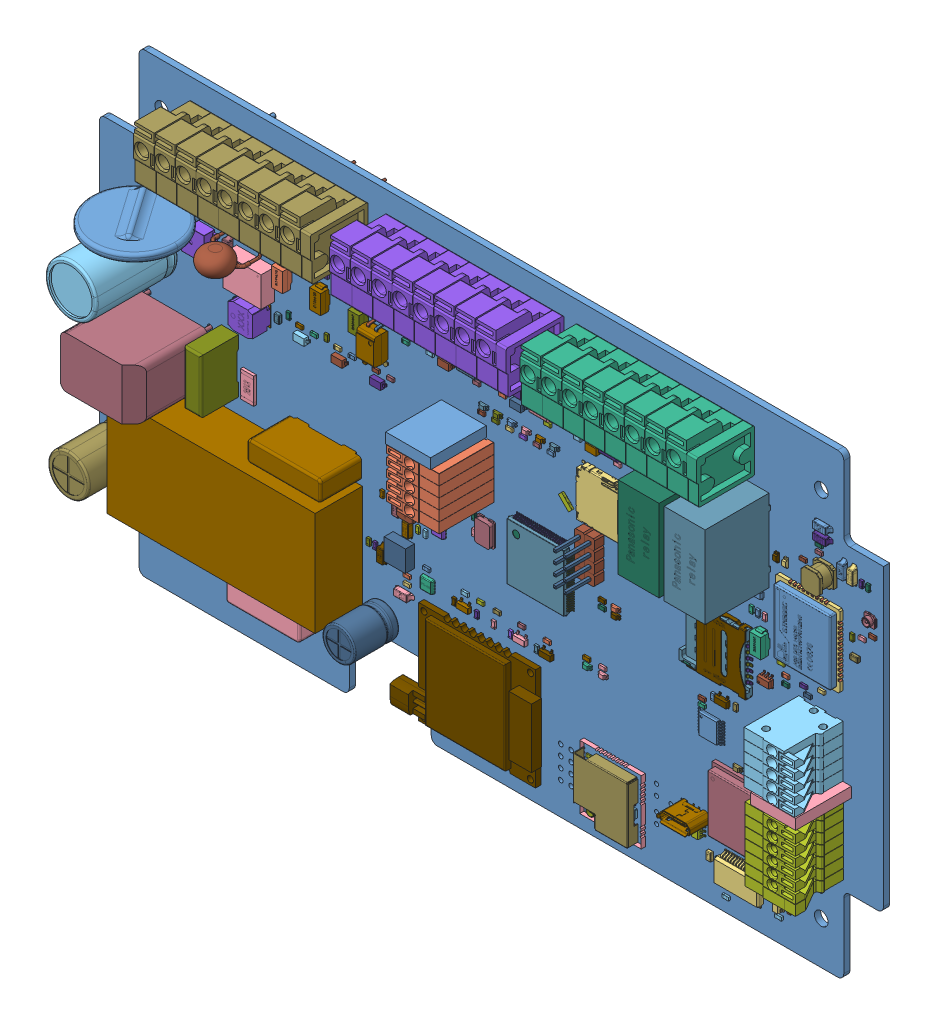
SolidWorks assembly Velvet_Controller_V1.2_2023, configuration Default. Lengths in mm.
Overall size (191.4 111.4 51.25).
933 component instances, 385 part files, 0 mates.
Components (placement in the parent):
- Velvet_Controller_V1.2_2023(2)^Velvet_Controller_V1.2_2023-1: Velvet_Controller_V1.2_2023(2)^Velvet_Controller_V1.2_2023 [Default] at origin size (191.4 111.4 51.25) (virtual)
  - Board^Velvet_Controller_V1.2_2023(2)_Velvet_Controller_V1.2_2023-1: Board^Velvet_Controller_V1.2_2023(2)_Velvet_Controller_V1.2_2023 [Default] at origin size (191.4 111.4 1.5) (virtual)
    - Open CASCADE STEP translator 7.5 1.1.1^Board_Velvet_Controller_V1.2_2023(2)_Velvet_Controller_V1.2_2023-1: Open CASCADE STEP translator 7.5 1.1.1^Board_Velvet_Controller_V1.2_2023(2)_Velvet_Controller_V1.2_2023 [Default] at (0 0 -1.5) size (215.4 111.4 1.5) (virtual)
  - VD21mc^Velvet_Controller_V1.2_2023(2)_Velvet_Controller_V1.2_2023-1: VD21mc^Velvet_Controller_V1.2_2023(2)_Velvet_Controller_V1.2_2023 [Default] at origin size (1 1.6 0.6) (virtual)
    - 6303145504^VD21mc_Velvet_Controller_V1.2_2023(2)_Velvet_Controller_V1.2_2023-1: 6303145504^VD21mc_Velvet_Controller_V1.2_2023(2)_Velvet_Controller_V1.2_2023 [Default] at (170 35.875 0) size (1 1.6 0.6) (virtual)
      - Extruded^6303145504_VD21mc_Velvet_Controller_V1.2_2023(2)_Velvet_Controller_V1.2_2023-1: Extruded^6303145504_VD21mc_Velvet_Controller_V1.2_2023(2)_Velvet_Controller_V1.2_2023 [Default] at origin size (1 1.6 0.6) (virtual)
  - VD20mc^Velvet_Controller_V1.2_2023(2)_Velvet_Controller_V1.2_2023-1: VD20mc^Velvet_Controller_V1.2_2023(2)_Velvet_Controller_V1.2_2023 [Default] at origin size (1 1.6 0.6) (virtual)
    - 6303145504^VD20mc_Velvet_Controller_V1.2_2023(2)_Velvet_Controller_V1.2_2023-1: 6303145504^VD20mc_Velvet_Controller_V1.2_2023(2)_Velvet_Controller_V1.2_2023 [Default] at (170 37.85 0) size (1 1.6 0.6) (virtual)
      - Extruded^6303145504_VD20mc_Velvet_Controller_V1.2_2023(2)_Velvet_Controller_V1.2_2023-1: Extruded^6303145504_VD20mc_Velvet_Controller_V1.2_2023(2)_Velvet_Controller_V1.2_2023 [Default] at origin size (1 1.6 0.6) (virtual)
  - VD19mc^Velvet_Controller_V1.2_2023(2)_Velvet_Controller_V1.2_2023-1: VD19mc^Velvet_Controller_V1.2_2023(2)_Velvet_Controller_V1.2_2023 [Default] at origin size (1 1.6 0.6) (virtual)
    - 6303145504^VD19mc_Velvet_Controller_V1.2_2023(2)_Velvet_Controller_V1.2_2023-1: 6303145504^VD19mc_Velvet_Controller_V1.2_2023(2)_Velvet_Controller_V1.2_2023 [Default] at (170 32.725 0) size (1 1.6 0.6) (virtual)
      - Extruded^6303145504_VD19mc_Velvet_Controller_V1.2_2023(2)_Velvet_Controller_V1.2_2023-1: Extruded^6303145504_VD19mc_Velvet_Controller_V1.2_2023(2)_Velvet_Controller_V1.2_2023 [Default] at origin size (1 1.6 0.6) (virtual)
  - VD18mc^Velvet_Controller_V1.2_2023(2)_Velvet_Controller_V1.2_2023-1: VD18mc^Velvet_Controller_V1.2_2023(2)_Velvet_Controller_V1.2_2023 [Default] at origin size (1 1.6 0.6) (virtual)
    - 6303145504^VD18mc_Velvet_Controller_V1.2_2023(2)_Velvet_Controller_V1.2_2023-1: 6303145504^VD18mc_Velvet_Controller_V1.2_2023(2)_Velvet_Controller_V1.2_2023 [Default] at (170 30.71 0) size (1 1.6 0.6) (virtual)
      - Extruded^6303145504_VD18mc_Velvet_Controller_V1.2_2023(2)_Velvet_Controller_V1.2_2023-1: Extruded^6303145504_VD18mc_Velvet_Controller_V1.2_2023(2)_Velvet_Controller_V1.2_2023 [Default] at origin size (1 1.6 0.6) (virtual)
  - VD17mc^Velvet_Controller_V1.2_2023(2)_Velvet_Controller_V1.2_2023-1: VD17mc^Velvet_Controller_V1.2_2023(2)_Velvet_Controller_V1.2_2023 [Default] at origin size (1 1.6 0.6) (virtual)
    - 6303145504^VD17mc_Velvet_Controller_V1.2_2023(2)_Velvet_Controller_V1.2_2023-1: 6303145504^VD17mc_Velvet_Controller_V1.2_2023(2)_Velvet_Controller_V1.2_2023 [Default] at (169.95 25.675 0) size (1 1.6 0.6) (virtual)
      - Extruded^6303145504_VD17mc_Velvet_Controller_V1.2_2023(2)_Velvet_Controller_V1.2_2023-1: Extruded^6303145504_VD17mc_Velvet_Controller_V1.2_2023(2)_Velvet_Controller_V1.2_2023 [Default] at origin size (1 1.6 0.6) (virtual)
  - DA1mc^Velvet_Controller_V1.2_2023(2)_Velvet_Controller_V1.2_2023-1: DA1mc^Velvet_Controller_V1.2_2023(2)_Velvet_Controller_V1.2_2023 [Default] at origin size (3.39 3.39 0.56) (virtual)
    - MICROQFN16_1P25X3P55X0P4_STM^DA1mc_Velvet_Controller_V1.2_2023(2)_Velvet_Controller_V1.2_2023-1: MICROQFN16_1P25X3P55X0P4_STM^DA1mc_Velvet_Controller_V1.2_2023(2)_Velvet_Controller_V1.2_2023 [Default] at (114.2132 67.6824 0) x (0.707107 0.707107 0) z (0 0 1) size (1.25 3.55 0.56) (virtual)
  - VD22io^Velvet_Controller_V1.2_2023(2)_Velvet_Controller_V1.2_2023-1: VD22io^Velvet_Controller_V1.2_2023(2)_Velvet_Controller_V1.2_2023 [Default] at origin size (3.7 1.6 1.15) (virtual)
    - SOD 123^VD22io_Velvet_Controller_V1.2_2023(2)_Velvet_Controller_V1.2_2023-1: SOD 123^VD22io_Velvet_Controller_V1.2_2023(2)_Velvet_Controller_V1.2_2023 [Default] at (138.2 82.5 0) x (1 0 0) z (0 0 1) size (3.7 1.6 1.15) (virtual)
  - VD21io^Velvet_Controller_V1.2_2023(2)_Velvet_Controller_V1.2_2023-1: VD21io^Velvet_Controller_V1.2_2023(2)_Velvet_Controller_V1.2_2023 [Default] at origin size (3.7 1.6 1.15) (virtual)
    - SOD 123^VD21io_Velvet_Controller_V1.2_2023(2)_Velvet_Controller_V1.2_2023-1: SOD 123^VD21io_Velvet_Controller_V1.2_2023(2)_Velvet_Controller_V1.2_2023 [Default] at (121 82.5 0) x (1 0 0) z (0 0 1) size (3.7 1.6 1.15) (virtual)
  - VD20io^Velvet_Controller_V1.2_2023(2)_Velvet_Controller_V1.2_2023-1: VD20io^Velvet_Controller_V1.2_2023(2)_Velvet_Controller_V1.2_2023 [Default] at origin size (3.7 1.6 1.15) (virtual)
    - SOD 123^VD20io_Velvet_Controller_V1.2_2023(2)_Velvet_Controller_V1.2_2023-1: SOD 123^VD20io_Velvet_Controller_V1.2_2023(2)_Velvet_Controller_V1.2_2023 [Default] at (102.635 82.5 0) x (1 0 0) z (0 0 1) size (3.7 1.6 1.15) (virtual)
  - VD19io^Velvet_Controller_V1.2_2023(2)_Velvet_Controller_V1.2_2023-1: VD19io^Velvet_Controller_V1.2_2023(2)_Velvet_Controller_V1.2_2023 [Default] at origin size (3.7 1.6 1.15) (virtual)
    - SOD 123^VD19io_Velvet_Controller_V1.2_2023(2)_Velvet_Controller_V1.2_2023-1: SOD 123^VD19io_Velvet_Controller_V1.2_2023(2)_Velvet_Controller_V1.2_2023 [Default] at (85.01 82.45 0) x (1 0 0) z (0 0 1) size (3.7 1.6 1.15) (virtual)
  - C5p^Velvet_Controller_V1.2_2023(2)_Velvet_Controller_V1.2_2023-1: C5p^Velvet_Controller_V1.2_2023(2)_Velvet_Controller_V1.2_2023 [Default] at origin size (10 10 33) (virtual)
    - ECA1HM331^C5p_Velvet_Controller_V1.2_2023(2)_Velvet_Controller_V1.2_2023-1: ECA1HM331^C5p_Velvet_Controller_V1.2_2023(2)_Velvet_Controller_V1.2_2023 [Default] at (8.4 28.2 0) x (0 1 0) z (1 0 0) size (10 33 10) (virtual)
  - ZQ1mc^Velvet_Controller_V1.2_2023(2)_Velvet_Controller_V1.2_2023-1: ZQ1mc^Velvet_Controller_V1.2_2023(2)_Velvet_Controller_V1.2_2023 [Default] at origin size (4.2 5.75 1.3) (virtual)
    - ABM3-8_000MHZ-D2Y-T_ABR^ZQ1mc_Velvet_Controller_V1.2_2023(2)_Velvet_Controller_V1.2_2023-1: ABM3-8_000MHZ-D2Y-T_ABR^ZQ1mc_Velvet_Controller_V1.2_2023(2)_Velvet_Controller_V1.2_2023 [Default] at (94.675 51.625 0) x (0 -1 0) z (0 0 1) size (5.75 4.2 1.3) (virtual)
  - XS1gs^Velvet_Controller_V1.2_2023(2)_Velvet_Controller_V1.2_2023-1: XS1gs^Velvet_Controller_V1.2_2023(2)_Velvet_Controller_V1.2_2023 [Default] at origin size (16.3 15.4 1.94) (virtual)
    - 693022010811 (rev1)^XS1gs_Velvet_Controller_V1.2_2023(2)_Velvet_Controller_V1.2_2023-1: 693022010811 (rev1)^XS1gs_Velvet_Controller_V1.2_2023(2)_Velvet_Controller_V1.2_2023 [Default] at (151.375 56.415 0.1) x (0 1 0) z (0 0 1) size (15.4 16.3 1.94) (virtual)
      - 693022010811^693022010811 (rev1)_XS1gs_Velvet_Controller_V1.2_2023(2)_Velvet_Controller_V1.2_2023-1: 693022010811^693022010811 (rev1)_XS1gs_Velvet_Controller_V1.2_2023(2)_Velvet_Controller_V1.2_2023 [Default] at origin size (14.66 16.3 1.75) (virtual)
      - 693022010811-0^693022010811 (rev1)_XS1gs_Velvet_Controller_V1.2_2023(2)_Velvet_Controller_V1.2_2023-1: 693022010811-0^693022010811 (rev1)_XS1gs_Velvet_Controller_V1.2_2023(2)_Velvet_Controller_V1.2_2023 [Default] at origin size (15.4 15.7 1.75) (virtual)
      - 693022010811_PIN_COURTE^693022010811 (rev1)_XS1gs_Velvet_Controller_V1.2_2023(2)_Velvet_Controller_V1.2_2023-1: 693022010811_PIN_COURTE^693022010811 (rev1)_XS1gs_Velvet_Controller_V1.2_2023(2)_Velvet_Controller_V1.2_2023 [Default] at (-3.75 -6.275 0.3) size (0.96 5.4 1.32) (virtual)
      - 693022010811_PIN_COURTE^693022010811 (rev1)_XS1gs_Velvet_Controller_V1.2_2023(2)_Velvet_Controller_V1.2_2023-2: 693022010811_PIN_COURTE^693022010811 (rev1)_XS1gs_Velvet_Controller_V1.2_2023(2)_Velvet_Controller_V1.2_2023 [Default] at (-1.21 -6.275 0.3) size (0.96 5.4 1.32) (virtual)
      - 693022010811_PIN_COURTE^693022010811 (rev1)_XS1gs_Velvet_Controller_V1.2_2023(2)_Velvet_Controller_V1.2_2023-3: 693022010811_PIN_COURTE^693022010811 (rev1)_XS1gs_Velvet_Controller_V1.2_2023(2)_Velvet_Controller_V1.2_2023 [Default] at (1.33 -6.275 0.3) size (0.96 5.4 1.32) (virtual)
      - 693022010811_PIN_COURTE^693022010811 (rev1)_XS1gs_Velvet_Controller_V1.2_2023(2)_Velvet_Controller_V1.2_2023-4: 693022010811_PIN_COURTE^693022010811 (rev1)_XS1gs_Velvet_Controller_V1.2_2023(2)_Velvet_Controller_V1.2_2023 [Default] at (3.87 -6.275 0.3) size (0.96 5.4 1.32) (virtual)
      - 693022010811_PIN_LONGUE^693022010811 (rev1)_XS1gs_Velvet_Controller_V1.2_2023(2)_Velvet_Controller_V1.2_2023-1: 693022010811_PIN_LONGUE^693022010811 (rev1)_XS1gs_Velvet_Controller_V1.2_2023(2)_Velvet_Controller_V1.2_2023 [Default] at (-4.16 0.05 0.3) size (1.9 12.4 1.32) (virtual)
      - 693022010811_PIN_LONGUE^693022010811 (rev1)_XS1gs_Velvet_Controller_V1.2_2023(2)_Velvet_Controller_V1.2_2023-2: 693022010811_PIN_LONGUE^693022010811 (rev1)_XS1gs_Velvet_Controller_V1.2_2023(2)_Velvet_Controller_V1.2_2023 [Default] at (-1.62 0.05 0.3) size (1.9 12.4 1.32) (virtual)
      - 693022010811_PIN_LONGUE^693022010811 (rev1)_XS1gs_Velvet_Controller_V1.2_2023(2)_Velvet_Controller_V1.2_2023-3: 693022010811_PIN_LONGUE^693022010811 (rev1)_XS1gs_Velvet_Controller_V1.2_2023(2)_Velvet_Controller_V1.2_2023 [Default] at (0.92 0.05 0.3) size (1.9 12.4 1.32) (virtual)
      - 693022010811_PIN_LONGUE^693022010811 (rev1)_XS1gs_Velvet_Controller_V1.2_2023(2)_Velvet_Controller_V1.2_2023-4: 693022010811_PIN_LONGUE^693022010811 (rev1)_XS1gs_Velvet_Controller_V1.2_2023(2)_Velvet_Controller_V1.2_2023 [Default] at (3.46 0.05 0.3) size (1.9 12.4 1.32) (virtual)
      - 693022010811_SHIELDING^693022010811 (rev1)_XS1gs_Velvet_Controller_V1.2_2023(2)_Velvet_Controller_V1.2_2023-1: 693022010811_SHIELDING^693022010811 (rev1)_XS1gs_Velvet_Controller_V1.2_2023(2)_Velvet_Controller_V1.2_2023 [Default] at (0 -0.7 1.645) size (14.86 14.9 1.65) (virtual)
  - X5mc^Velvet_Controller_V1.2_2023(2)_Velvet_Controller_V1.2_2023-1: X5mc^Velvet_Controller_V1.2_2023(2)_Velvet_Controller_V1.2_2023 [Default] at origin size (12.8 15.3 17.1) (virtual)
    - 7243191056^X5mc_Velvet_Controller_V1.2_2023(2)_Velvet_Controller_V1.2_2023-1: 7243191056^X5mc_Velvet_Controller_V1.2_2023(2)_Velvet_Controller_V1.2_2023 [Default] at (88.9525 72.425 0) size (10.96 2.54 13.6) (virtual)
      - Extruded-1^7243191056_X5mc_Velvet_Controller_V1.2_2023(2)_Velvet_Controller_V1.2_2023-1: Extruded-1^7243191056_X5mc_Velvet_Controller_V1.2_2023(2)_Velvet_Controller_V1.2_2023 [Default] at origin size (10.96 2.54 13.6) (virtual)
    - DG141V^X5mc_Velvet_Controller_V1.2_2023(2)_Velvet_Controller_V1.2_2023-1: DG141V^X5mc_Velvet_Controller_V1.2_2023(2)_Velvet_Controller_V1.2_2023 [Default] at (89.975 58.395 0) x (-1 0 0) z (0 0 -1) size (12.6 2.63 17.1) (virtual)
    - DG141V^X5mc_Velvet_Controller_V1.2_2023(2)_Velvet_Controller_V1.2_2023-2: DG141V^X5mc_Velvet_Controller_V1.2_2023(2)_Velvet_Controller_V1.2_2023 [Default] at (89.975 60.935 0) x (-1 0 0) z (0 0 -1) size (12.6 2.63 17.1) (virtual)
    - DG141V^X5mc_Velvet_Controller_V1.2_2023(2)_Velvet_Controller_V1.2_2023-3: DG141V^X5mc_Velvet_Controller_V1.2_2023(2)_Velvet_Controller_V1.2_2023 [Default] at (89.975 63.475 0) x (-1 0 0) z (0 0 -1) size (12.6 2.63 17.1) (virtual)
    - DG141V^X5mc_Velvet_Controller_V1.2_2023(2)_Velvet_Controller_V1.2_2023-4: DG141V^X5mc_Velvet_Controller_V1.2_2023(2)_Velvet_Controller_V1.2_2023 [Default] at (89.975 66.015 0) x (-1 0 0) z (0 0 -1) size (12.6 2.63 17.1) (virtual)
    - DG141V^X5mc_Velvet_Controller_V1.2_2023(2)_Velvet_Controller_V1.2_2023-5: DG141V^X5mc_Velvet_Controller_V1.2_2023(2)_Velvet_Controller_V1.2_2023 [Default] at (89.975 68.555 0) x (-1 0 0) z (0 0 -1) size (12.6 2.63 17.1) (virtual)
  - X4mc^Velvet_Controller_V1.2_2023(2)_Velvet_Controller_V1.2_2023-1: X4mc^Velvet_Controller_V1.2_2023(2)_Velvet_Controller_V1.2_2023 [Default] at origin size (11.5 11.95 1.68) (virtual)
    - 114-00841-68^X4mc_Velvet_Controller_V1.2_2023(2)_Velvet_Controller_V1.2_2023-1: 114-00841-68^X4mc_Velvet_Controller_V1.2_2023(2)_Velvet_Controller_V1.2_2023 [Default] at (123.675 72.425 0) x (0 1 0) z (1 0 0) size (11.95 1.68 11.5) (virtual)
  - X3mc^Velvet_Controller_V1.2_2023(2)_Velvet_Controller_V1.2_2023-1: X3mc^Velvet_Controller_V1.2_2023(2)_Velvet_Controller_V1.2_2023 [Default] at origin size (12.8 15.3 17.1) (virtual)
    - 7243191056^X3mc_Velvet_Controller_V1.2_2023(2)_Velvet_Controller_V1.2_2023-1: 7243191056^X3mc_Velvet_Controller_V1.2_2023(2)_Velvet_Controller_V1.2_2023 [Default] at (178.0475 40.74 0) size (10.96 2.54 13.6) (virtual)
      - Extruded-1^7243191056_X3mc_Velvet_Controller_V1.2_2023(2)_Velvet_Controller_V1.2_2023-1: Extruded-1^7243191056_X3mc_Velvet_Controller_V1.2_2023(2)_Velvet_Controller_V1.2_2023 [Default] at origin size (10.96 2.54 13.6) (virtual)
    - DG141V^X3mc_Velvet_Controller_V1.2_2023(2)_Velvet_Controller_V1.2_2023-1: DG141V^X3mc_Velvet_Controller_V1.2_2023(2)_Velvet_Controller_V1.2_2023 [Default] at (177.025 54.77 0) x (1 0 0) z (0 0 -1) size (12.6 2.63 17.1) (virtual)
    - DG141V^X3mc_Velvet_Controller_V1.2_2023(2)_Velvet_Controller_V1.2_2023-2: DG141V^X3mc_Velvet_Controller_V1.2_2023(2)_Velvet_Controller_V1.2_2023 [Default] at (177.025 52.23 0) x (1 0 0) z (0 0 -1) size (12.6 2.63 17.1) (virtual)
    - DG141V^X3mc_Velvet_Controller_V1.2_2023(2)_Velvet_Controller_V1.2_2023-3: DG141V^X3mc_Velvet_Controller_V1.2_2023(2)_Velvet_Controller_V1.2_2023 [Default] at (177.025 49.69 0) x (1 0 0) z (0 0 -1) size (12.6 2.63 17.1) (virtual)
    - DG141V^X3mc_Velvet_Controller_V1.2_2023(2)_Velvet_Controller_V1.2_2023-4: DG141V^X3mc_Velvet_Controller_V1.2_2023(2)_Velvet_Controller_V1.2_2023 [Default] at (177.025 47.15 0) x (1 0 0) z (0 0 -1) size (12.6 2.63 17.1) (virtual)
    - DG141V^X3mc_Velvet_Controller_V1.2_2023(2)_Velvet_Controller_V1.2_2023-5: DG141V^X3mc_Velvet_Controller_V1.2_2023(2)_Velvet_Controller_V1.2_2023 [Default] at (177.025 44.61 0) x (1 0 0) z (0 0 -1) size (12.6 2.63 17.1) (virtual)
  - X3io^Velvet_Controller_V1.2_2023(2)_Velvet_Controller_V1.2_2023-1: X3io^Velvet_Controller_V1.2_2023(2)_Velvet_Controller_V1.2_2023 [Default] at origin size (43.18 13.2 17.6) (virtual)
    - DG142V-8-5.08^X3io_Velvet_Controller_V1.2_2023(2)_Velvet_Controller_V1.2_2023-1: DG142V-8-5.08^X3io_Velvet_Controller_V1.2_2023(2)_Velvet_Controller_V1.2_2023 [Default] at (159.905 109.08 0) x (-1 0 0) z (0 1 0) size (43.18 17.6 13.2) (virtual)
  - X2mc^Velvet_Controller_V1.2_2023(2)_Velvet_Controller_V1.2_2023-1: X2mc^Velvet_Controller_V1.2_2023(2)_Velvet_Controller_V1.2_2023 [Default] at origin size (12.6 17.78 17.1) (virtual)
    - DG141V-5-2.54^X2mc_Velvet_Controller_V1.2_2023(2)_Velvet_Controller_V1.2_2023-1: DG141V-5-2.54^X2mc_Velvet_Controller_V1.2_2023(2)_Velvet_Controller_V1.2_2023 [Default] at (183.455 21.255 0) x (0 1 0) z (1 0 0) size (17.78 17.1 12.6) (virtual)
  - X2io^Velvet_Controller_V1.2_2023(2)_Velvet_Controller_V1.2_2023-1: X2io^Velvet_Controller_V1.2_2023(2)_Velvet_Controller_V1.2_2023 [Default] at origin size (43.18 13.2 17.6) (virtual)
    - DG142V-8-5.08^X2io_Velvet_Controller_V1.2_2023(2)_Velvet_Controller_V1.2_2023-1: DG142V-8-5.08^X2io_Velvet_Controller_V1.2_2023(2)_Velvet_Controller_V1.2_2023 [Default] at (113.405 109.08 0) x (-1 0 0) z (0 1 0) size (43.18 17.6 13.2) (virtual)
  - X1wf^Velvet_Controller_V1.2_2023(2)_Velvet_Controller_V1.2_2023-1: X1wf^Velvet_Controller_V1.2_2023(2)_Velvet_Controller_V1.2_2023 [Default] at origin size (7.94 2.84 7.9) (virtual)
    - USB3131-30-0230-A--3DModel-STEP-56544^X1wf_Velvet_Controller_V1.2_2023(2)_Velvet_Controller_V1.2_2023-1: USB3131-30-0230-A--3DModel-STEP-56544^X1wf_Velvet_Controller_V1.2_2023(2)_Velvet_Controller_V1.2_2023 [Default] at (145.7502 18.1395 -2) x (-1 0 0) z (0 1 0) size (7.94 7.9 2.84) (virtual)
  - X1mc^Velvet_Controller_V1.2_2023(2)_Velvet_Controller_V1.2_2023-1: X1mc^Velvet_Controller_V1.2_2023(2)_Velvet_Controller_V1.2_2023 [Default] at origin size (4.98 10.16 11.54) (virtual)
    - 2_54mm Male Header (4x2)^X1mc_Velvet_Controller_V1.2_2023(2)_Velvet_Controller_V1.2_2023-1: 2_54mm Male Header (4x2)^X1mc_Velvet_Controller_V1.2_2023(2)_Velvet_Controller_V1.2_2023 [Default] at (120.0963 91.9162 -15.24) x (0 1 0) z (0 0 1) size (10.16 4.98 11.54) (virtual)
      - User Library-Header_Male_4Pin^2_54mm Male Header (4x2)_X1mc_Velvet_Controller_V1.2_2023(2)_Velvet_Controller_V1.2_2023-1: User Library-Header_Male_4Pin^2_54mm Male Header (4x2)_X1mc_Velvet_Controller_V1.2_2023(2)_Velvet_Controller_V1.2_2023 [Default] at (-35.6012 -1.8987 15.2958) size (10.16 2.49 11.54) (virtual)
        - User Library-Header_Male_4Pin_PinArray^User Library-Header_Male_4Pin_2_54mm Male Header (4x2)_X1mc_Velvet_Controller_V1.2_2023(2)_Velvet_Controller_V1.2_2023-1: User Library-Header_Male_4Pin_PinArray^User Library-Header_Male_4Pin_2_54mm Male Header (4x2)_X1mc_Velvet_Controller_V1.2_2023(2)_Velvet_Controller_V1.2_2023 [Default] at origin size (8.26 0.64 11.54) (virtual)
        - User Library-Header_Male_4Pin_BodyArray^User Library-Header_Male_4Pin_2_54mm Male Header (4x2)_X1mc_Velvet_Controller_V1.2_2023(2)_Velvet_Controller_V1.2_2023-1: User Library-Header_Male_4Pin_BodyArray^User Library-Header_Male_4Pin_2_54mm Male Header (4x2)_X1mc_Velvet_Controller_V1.2_2023(2)_Velvet_Controller_V1.2_2023 [Default] at origin size (10.16 2.49 2.29) (virtual)
      - User Library-Header_Male_4Pin^2_54mm Male Header (4x2)_X1mc_Velvet_Controller_V1.2_2023(2)_Velvet_Controller_V1.2_2023-2: User Library-Header_Male_4Pin^2_54mm Male Header (4x2)_X1mc_Velvet_Controller_V1.2_2023(2)_Velvet_Controller_V1.2_2023 [Default] at (-35.6012 0.5913 15.2958) size (10.16 2.49 11.54) (virtual)
        - User Library-Header_Male_4Pin_PinArray^User Library-Header_Male_4Pin_2_54mm Male Header (4x2)_X1mc_Velvet_Controller_V1.2_2023(2)_Velvet_Controller_V1.2_2023-1: User Library-Header_Male_4Pin_PinArray^User Library-Header_Male_4Pin_2_54mm Male Header (4x2)_X1mc_Velvet_Controller_V1.2_2023(2)_Velvet_Controller_V1.2_2023 [Default] at origin size (8.26 0.64 11.54) (virtual)
        - User Library-Header_Male_4Pin_BodyArray^User Library-Header_Male_4Pin_2_54mm Male Header (4x2)_X1mc_Velvet_Controller_V1.2_2023(2)_Velvet_Controller_V1.2_2023-1: User Library-Header_Male_4Pin_BodyArray^User Library-Header_Male_4Pin_2_54mm Male Header (4x2)_X1mc_Velvet_Controller_V1.2_2023(2)_Velvet_Controller_V1.2_2023 [Default] at origin size (10.16 2.49 2.29) (virtual)
  - X1lr^Velvet_Controller_V1.2_2023(2)_Velvet_Controller_V1.2_2023-1: X1lr^Velvet_Controller_V1.2_2023(2)_Velvet_Controller_V1.2_2023 [Default] at origin (virtual)
    - 2_54mm Male Header (4x2).step-1: 2_54mm Male Header (4x2).step [Default] at (114.5837 -20.1153 -15.24) x (0 -1 0) z (0 0 1) (suppressed, hidden)
  - X1io^Velvet_Controller_V1.2_2023(2)_Velvet_Controller_V1.2_2023-1: X1io^Velvet_Controller_V1.2_2023(2)_Velvet_Controller_V1.2_2023 [Default] at origin size (43.18 13.2 17.6) (virtual)
    - DG142V-8-5.08^X1io_Velvet_Controller_V1.2_2023(2)_Velvet_Controller_V1.2_2023-1: DG142V-8-5.08^X1io_Velvet_Controller_V1.2_2023(2)_Velvet_Controller_V1.2_2023 [Default] at (65.585 109.1 0) x (-1 0 0) z (0 1 0) size (43.18 17.6 13.2) (virtual)
  - X1gs^Velvet_Controller_V1.2_2023(2)_Velvet_Controller_V1.2_2023-1: X1gs^Velvet_Controller_V1.2_2023(2)_Velvet_Controller_V1.2_2023 [Default] at origin size (3 3.1 1.23) (virtual)
    - c-1909763-1-b-3d^X1gs_Velvet_Controller_V1.2_2023(2)_Velvet_Controller_V1.2_2023-1: c-1909763-1-b-3d^X1gs_Velvet_Controller_V1.2_2023(2)_Velvet_Controller_V1.2_2023 [Default] at (188.275 79.6 1.25) x (1 0 0) z (0 0 1) size (3 3.1 1.23) (virtual)
  - VT6io^Velvet_Controller_V1.2_2023(2)_Velvet_Controller_V1.2_2023-1: VT6io^Velvet_Controller_V1.2_2023(2)_Velvet_Controller_V1.2_2023 [Default] at origin size (3.45 3.45 0.82) (virtual)
    - PDFN33^VT6io_Velvet_Controller_V1.2_2023(2)_Velvet_Controller_V1.2_2023-1: PDFN33^VT6io_Velvet_Controller_V1.2_2023(2)_Velvet_Controller_V1.2_2023 [Default] at (136.075 85.725 0) x (0 1 0) z (0 0 1) size (3.45 3.45 0.82) (virtual)
  - VT5io^Velvet_Controller_V1.2_2023(2)_Velvet_Controller_V1.2_2023-1: VT5io^Velvet_Controller_V1.2_2023(2)_Velvet_Controller_V1.2_2023 [Default] at origin size (3.45 3.45 0.82) (virtual)
    - PDFN33^VT5io_Velvet_Controller_V1.2_2023(2)_Velvet_Controller_V1.2_2023-1: PDFN33^VT5io_Velvet_Controller_V1.2_2023(2)_Velvet_Controller_V1.2_2023 [Default] at (119.05 85.725 0) x (0 1 0) z (0 0 1) size (3.45 3.45 0.82) (virtual)
  - VT4lr^Velvet_Controller_V1.2_2023(2)_Velvet_Controller_V1.2_2023-1: VT4lr^Velvet_Controller_V1.2_2023(2)_Velvet_Controller_V1.2_2023 [Default] at origin size (2.92 2.48 1.02) (virtual)
    - SOT23-3^VT4lr_Velvet_Controller_V1.2_2023(2)_Velvet_Controller_V1.2_2023-1: SOT23-3^VT4lr_Velvet_Controller_V1.2_2023(2)_Velvet_Controller_V1.2_2023 [Default] at (109.85 26.9 -1.87) x (1 0 0) z (0 1 0) size (2.92 1.02 2.48) (virtual)
  - VT4io^Velvet_Controller_V1.2_2023(2)_Velvet_Controller_V1.2_2023-1: VT4io^Velvet_Controller_V1.2_2023(2)_Velvet_Controller_V1.2_2023 [Default] at origin size (3.45 3.45 0.82) (virtual)
    - PDFN33^VT4io_Velvet_Controller_V1.2_2023(2)_Velvet_Controller_V1.2_2023-1: PDFN33^VT4io_Velvet_Controller_V1.2_2023(2)_Velvet_Controller_V1.2_2023 [Default] at (101.95 85.7 0) x (0 1 0) z (0 0 1) size (3.45 3.45 0.82) (virtual)
  - VT3lr^Velvet_Controller_V1.2_2023(2)_Velvet_Controller_V1.2_2023-1: VT3lr^Velvet_Controller_V1.2_2023(2)_Velvet_Controller_V1.2_2023 [Default] at origin size (2.92 2.48 1.02) (virtual)
    - SOT23-3^VT3lr_Velvet_Controller_V1.2_2023(2)_Velvet_Controller_V1.2_2023-1: SOT23-3^VT3lr_Velvet_Controller_V1.2_2023(2)_Velvet_Controller_V1.2_2023 [Default] at (109.6 33.1 0.37) x (-1 0 0) z (0 1 0) size (2.92 1.02 2.48) (virtual)
  - VT3io^Velvet_Controller_V1.2_2023(2)_Velvet_Controller_V1.2_2023-1: VT3io^Velvet_Controller_V1.2_2023(2)_Velvet_Controller_V1.2_2023 [Default] at origin size (2.92 2.48 1.02) (virtual)
    - SOT23-3^VT3io_Velvet_Controller_V1.2_2023(2)_Velvet_Controller_V1.2_2023-1: SOT23-3^VT3io_Velvet_Controller_V1.2_2023(2)_Velvet_Controller_V1.2_2023 [Default] at (160.825 71.9 0.37) x (1 0 0) z (0 -1 0) size (2.92 1.02 2.48) (virtual)
  - VT3gs^Velvet_Controller_V1.2_2023(2)_Velvet_Controller_V1.2_2023-1: VT3gs^Velvet_Controller_V1.2_2023(2)_Velvet_Controller_V1.2_2023 [Default] at origin size (2.92 2.48 1.02) (virtual)
    - SOT23-3^VT3gs_Velvet_Controller_V1.2_2023(2)_Velvet_Controller_V1.2_2023-1: SOT23-3^VT3gs_Velvet_Controller_V1.2_2023(2)_Velvet_Controller_V1.2_2023 [Default] at (171.85 73.425 -1.87) x (-1 0 0) z (0 -1 0) size (2.92 1.02 2.48) (virtual)
  - VT2wf^Velvet_Controller_V1.2_2023(2)_Velvet_Controller_V1.2_2023-1: VT2wf^Velvet_Controller_V1.2_2023(2)_Velvet_Controller_V1.2_2023 [Default] at origin size (2.48 2.92 1.02) (virtual)
    - SOT23-3^VT2wf_Velvet_Controller_V1.2_2023(2)_Velvet_Controller_V1.2_2023-1: SOT23-3^VT2wf_Velvet_Controller_V1.2_2023(2)_Velvet_Controller_V1.2_2023 [Default] at (165.95 8.425 0.37) x (0 1 0) z (1 0 0) size (2.92 1.02 2.48) (virtual)
  - VT2lr^Velvet_Controller_V1.2_2023(2)_Velvet_Controller_V1.2_2023-1: VT2lr^Velvet_Controller_V1.2_2023(2)_Velvet_Controller_V1.2_2023 [Default] at origin size (2.92 2.48 1.02) (virtual)
    - SOT23-3^VT2lr_Velvet_Controller_V1.2_2023(2)_Velvet_Controller_V1.2_2023-1: SOT23-3^VT2lr_Velvet_Controller_V1.2_2023(2)_Velvet_Controller_V1.2_2023 [Default] at (103.3 33.1 0.37) x (-1 0 0) z (0 1 0) size (2.92 1.02 2.48) (virtual)
  - VT2io^Velvet_Controller_V1.2_2023(2)_Velvet_Controller_V1.2_2023-1: VT2io^Velvet_Controller_V1.2_2023(2)_Velvet_Controller_V1.2_2023 [Default] at origin size (3.45 3.45 0.82) (virtual)
    - PDFN33^VT2io_Velvet_Controller_V1.2_2023(2)_Velvet_Controller_V1.2_2023-1: PDFN33^VT2io_Velvet_Controller_V1.2_2023(2)_Velvet_Controller_V1.2_2023 [Default] at (84.65 85.5 0) x (0 1 0) z (0 0 1) size (3.45 3.45 0.82) (virtual)
  - VT2gs^Velvet_Controller_V1.2_2023(2)_Velvet_Controller_V1.2_2023-1: VT2gs^Velvet_Controller_V1.2_2023(2)_Velvet_Controller_V1.2_2023 [Default] at origin size (2.92 2.48 1.02) (virtual)
    - SOT23-3^VT2gs_Velvet_Controller_V1.2_2023(2)_Velvet_Controller_V1.2_2023-1: SOT23-3^VT2gs_Velvet_Controller_V1.2_2023(2)_Velvet_Controller_V1.2_2023 [Default] at (165.1 78.15 -1.87) x (-1 0 0) z (0 -1 0) size (2.92 1.02 2.48) (virtual)
  - VT1wf^Velvet_Controller_V1.2_2023(2)_Velvet_Controller_V1.2_2023-1: VT1wf^Velvet_Controller_V1.2_2023(2)_Velvet_Controller_V1.2_2023 [Default] at origin size (2.48 2.92 1.02) (virtual)
    - SOT23-3^VT1wf_Velvet_Controller_V1.2_2023(2)_Velvet_Controller_V1.2_2023-1: SOT23-3^VT1wf_Velvet_Controller_V1.2_2023(2)_Velvet_Controller_V1.2_2023 [Default] at (165.95 11.95 0.37) x (0 -1 0) z (-1 0 0) size (2.92 1.02 2.48) (virtual)
  - VT1p^Velvet_Controller_V1.2_2023(2)_Velvet_Controller_V1.2_2023-1: VT1p^Velvet_Controller_V1.2_2023(2)_Velvet_Controller_V1.2_2023 [Default] at origin size (9.7 6.58 2.3) (virtual)
    - TO-252^VT1p_Velvet_Controller_V1.2_2023(2)_Velvet_Controller_V1.2_2023-1: TO-252^VT1p_Velvet_Controller_V1.2_2023(2)_Velvet_Controller_V1.2_2023 [Default] at (25.075 78.7 0) x (0 1 0) z (1 0 0) size (6.58 2.3 9.7) (virtual)
  - VT1lr^Velvet_Controller_V1.2_2023(2)_Velvet_Controller_V1.2_2023-1: VT1lr^Velvet_Controller_V1.2_2023(2)_Velvet_Controller_V1.2_2023 [Default] at origin size (2.92 2.48 1.02) (virtual)
    - SOT23-3^VT1lr_Velvet_Controller_V1.2_2023(2)_Velvet_Controller_V1.2_2023-1: SOT23-3^VT1lr_Velvet_Controller_V1.2_2023(2)_Velvet_Controller_V1.2_2023 [Default] at (89.5 33.1 0.37) x (-1 0 0) z (0 1 0) size (2.92 1.02 2.48) (virtual)
  - VT1io^Velvet_Controller_V1.2_2023(2)_Velvet_Controller_V1.2_2023-1: VT1io^Velvet_Controller_V1.2_2023(2)_Velvet_Controller_V1.2_2023 [Default] at origin size (2.92 2.48 1.02) (virtual)
    - SOT23-3^VT1io_Velvet_Controller_V1.2_2023(2)_Velvet_Controller_V1.2_2023-1: SOT23-3^VT1io_Velvet_Controller_V1.2_2023(2)_Velvet_Controller_V1.2_2023 [Default] at (149.425 71.95 0.37) x (1 0 0) z (0 -1 0) size (2.92 1.02 2.48) (virtual)
  - VT1gs^Velvet_Controller_V1.2_2023(2)_Velvet_Controller_V1.2_2023-1: VT1gs^Velvet_Controller_V1.2_2023(2)_Velvet_Controller_V1.2_2023 [Default] at origin size (2.92 2.48 1.02) (virtual)
    - SOT23-3^VT1gs_Velvet_Controller_V1.2_2023(2)_Velvet_Controller_V1.2_2023-1: SOT23-3^VT1gs_Velvet_Controller_V1.2_2023(2)_Velvet_Controller_V1.2_2023 [Default] at (168.35 78.125 -1.87) x (-1 0 0) z (0 -1 0) size (2.92 1.02 2.48) (virtual)
  - VD18io^Velvet_Controller_V1.2_2023(2)_Velvet_Controller_V1.2_2023-1: VD18io^Velvet_Controller_V1.2_2023(2)_Velvet_Controller_V1.2_2023 [Default] at origin size (8.13 6.11 2.39) (virtual)
    - DO214-AB (SOC)^VD18io_Velvet_Controller_V1.2_2023(2)_Velvet_Controller_V1.2_2023-1: DO214-AB (SOC)^VD18io_Velvet_Controller_V1.2_2023(2)_Velvet_Controller_V1.2_2023 [Default] at (136.25 90.925 0) x (1 0 0) z (0 0 1) size (8.13 6.11 2.39) (virtual)
  - VD17io^Velvet_Controller_V1.2_2023(2)_Velvet_Controller_V1.2_2023-1: VD17io^Velvet_Controller_V1.2_2023(2)_Velvet_Controller_V1.2_2023 [Default] at origin size (8.13 6.11 2.39) (virtual)
    - DO214-AB (SOC)^VD17io_Velvet_Controller_V1.2_2023(2)_Velvet_Controller_V1.2_2023-1: DO214-AB (SOC)^VD17io_Velvet_Controller_V1.2_2023(2)_Velvet_Controller_V1.2_2023 [Default] at (119.25 90.925 0) x (1 0 0) z (0 0 1) size (8.13 6.11 2.39) (virtual)
  - VD16mc^Velvet_Controller_V1.2_2023(2)_Velvet_Controller_V1.2_2023-1: VD16mc^Velvet_Controller_V1.2_2023(2)_Velvet_Controller_V1.2_2023 [Default] at origin size (1 1.6 0.6) (virtual)
    - 6303145504^VD16mc_Velvet_Controller_V1.2_2023(2)_Velvet_Controller_V1.2_2023-1: 6303145504^VD16mc_Velvet_Controller_V1.2_2023(2)_Velvet_Controller_V1.2_2023 [Default] at (169.95 27.685 0) size (1 1.6 0.6) (virtual)
      - Extruded^6303145504_VD16mc_Velvet_Controller_V1.2_2023(2)_Velvet_Controller_V1.2_2023-1: Extruded^6303145504_VD16mc_Velvet_Controller_V1.2_2023(2)_Velvet_Controller_V1.2_2023 [Default] at origin size (1 1.6 0.6) (virtual)
  - VD16io^Velvet_Controller_V1.2_2023(2)_Velvet_Controller_V1.2_2023-1: VD16io^Velvet_Controller_V1.2_2023(2)_Velvet_Controller_V1.2_2023 [Default] at origin size (2.48 2.92 1.02) (virtual)
    - SOT23-3^VD16io_Velvet_Controller_V1.2_2023(2)_Velvet_Controller_V1.2_2023-1: SOT23-3^VD16io_Velvet_Controller_V1.2_2023(2)_Velvet_Controller_V1.2_2023 [Default] at (67.9 87.2 0.37) x (0 -1 0) z (-1 0 0) size (2.92 1.02 2.48) (virtual)
  - VD15mc^Velvet_Controller_V1.2_2023(2)_Velvet_Controller_V1.2_2023-1: VD15mc^Velvet_Controller_V1.2_2023(2)_Velvet_Controller_V1.2_2023 [Default] at origin (virtual)
    - 6303145504.step-1: 6303145504.step [Default] at (157.975 45.675 0) (suppressed, hidden)
  - VD15io^Velvet_Controller_V1.2_2023(2)_Velvet_Controller_V1.2_2023-1: VD15io^Velvet_Controller_V1.2_2023(2)_Velvet_Controller_V1.2_2023 [Default] at origin size (2.79 5.49 2.29) (virtual)
    - DO-214AC(SMA)-2^VD15io_Velvet_Controller_V1.2_2023(2)_Velvet_Controller_V1.2_2023-1: DO-214AC(SMA)-2^VD15io_Velvet_Controller_V1.2_2023(2)_Velvet_Controller_V1.2_2023 [Default] at (64.28 81.3 0) x (0 1 0) z (1 0 0) size (5.49 2.29 2.79) (virtual)
  - VD14mc^Velvet_Controller_V1.2_2023(2)_Velvet_Controller_V1.2_2023-1: VD14mc^Velvet_Controller_V1.2_2023(2)_Velvet_Controller_V1.2_2023 [Default] at origin (virtual)
    - 6303145504.step-1: 6303145504.step [Default] at (157.975 43.45 0) (suppressed, hidden)
  - VD14io^Velvet_Controller_V1.2_2023(2)_Velvet_Controller_V1.2_2023-1: VD14io^Velvet_Controller_V1.2_2023(2)_Velvet_Controller_V1.2_2023 [Default] at origin size (3.7 1.6 1.15) (virtual)
    - SOD 123^VD14io_Velvet_Controller_V1.2_2023(2)_Velvet_Controller_V1.2_2023-1: SOD 123^VD14io_Velvet_Controller_V1.2_2023(2)_Velvet_Controller_V1.2_2023 [Default] at (68.38 70.1 0) x (1 0 0) z (0 0 1) size (3.7 1.6 1.15) (virtual)
  - VD13mc^Velvet_Controller_V1.2_2023(2)_Velvet_Controller_V1.2_2023-1: VD13mc^Velvet_Controller_V1.2_2023(2)_Velvet_Controller_V1.2_2023 [Default] at origin size (2.06 0.91 0.84) (virtual)
    - LED 0805^VD13mc_Velvet_Controller_V1.2_2023(2)_Velvet_Controller_V1.2_2023-1: LED 0805^VD13mc_Velvet_Controller_V1.2_2023(2)_Velvet_Controller_V1.2_2023 [Default] at (127.0968 49.6 0) x (0 -1 0) z (0 0 1) size (0.91 2.06 0.84) (virtual)
  - VD13io^Velvet_Controller_V1.2_2023(2)_Velvet_Controller_V1.2_2023-1: VD13io^Velvet_Controller_V1.2_2023(2)_Velvet_Controller_V1.2_2023 [Default] at origin size (5.49 2.79 2.29) (virtual)
    - DO-214AC(SMA)-2^VD13io_Velvet_Controller_V1.2_2023(2)_Velvet_Controller_V1.2_2023-1: DO-214AC(SMA)-2^VD13io_Velvet_Controller_V1.2_2023(2)_Velvet_Controller_V1.2_2023 [Default] at (65.4 91.3 0) x (-1 0 0) z (0 1 0) size (5.49 2.29 2.79) (virtual)
  - VD12mc^Velvet_Controller_V1.2_2023(2)_Velvet_Controller_V1.2_2023-1: VD12mc^Velvet_Controller_V1.2_2023(2)_Velvet_Controller_V1.2_2023 [Default] at origin size (2.06 0.91 0.84) (virtual)
    - LED 0805^VD12mc_Velvet_Controller_V1.2_2023(2)_Velvet_Controller_V1.2_2023-1: LED 0805^VD12mc_Velvet_Controller_V1.2_2023(2)_Velvet_Controller_V1.2_2023 [Default] at (127.0974 51.1319 0) x (0 -1 0) z (0 0 1) size (0.91 2.06 0.84) (virtual)
  - VD12io^Velvet_Controller_V1.2_2023(2)_Velvet_Controller_V1.2_2023-1: VD12io^Velvet_Controller_V1.2_2023(2)_Velvet_Controller_V1.2_2023 [Default] at origin size (8.13 6.11 2.39) (virtual)
    - DO214-AB (SOC)^VD12io_Velvet_Controller_V1.2_2023(2)_Velvet_Controller_V1.2_2023-1: DO214-AB (SOC)^VD12io_Velvet_Controller_V1.2_2023(2)_Velvet_Controller_V1.2_2023 [Default] at (101.885 90.925 0) x (1 0 0) z (0 0 1) size (8.13 6.11 2.39) (virtual)
  - VD11mc^Velvet_Controller_V1.2_2023(2)_Velvet_Controller_V1.2_2023-1: VD11mc^Velvet_Controller_V1.2_2023(2)_Velvet_Controller_V1.2_2023 [Default] at origin size (2.06 0.91 0.84) (virtual)
    - LED 0805^VD11mc_Velvet_Controller_V1.2_2023(2)_Velvet_Controller_V1.2_2023-1: LED 0805^VD11mc_Velvet_Controller_V1.2_2023(2)_Velvet_Controller_V1.2_2023 [Default] at (122.455 35.472 0) x (0 1 0) z (0 0 1) size (0.91 2.06 0.84) (virtual)
  - VD11io^Velvet_Controller_V1.2_2023(2)_Velvet_Controller_V1.2_2023-1: VD11io^Velvet_Controller_V1.2_2023(2)_Velvet_Controller_V1.2_2023 [Default] at origin size (2.48 2.92 1.02) (virtual)
    - SOT23-3^VD11io_Velvet_Controller_V1.2_2023(2)_Velvet_Controller_V1.2_2023-1: SOT23-3^VD11io_Velvet_Controller_V1.2_2023(2)_Velvet_Controller_V1.2_2023 [Default] at (58.6 87.3 0.37) x (0 -1 0) z (-1 0 0) size (2.92 1.02 2.48) (virtual)
  - VD10mc^Velvet_Controller_V1.2_2023(2)_Velvet_Controller_V1.2_2023-1: VD10mc^Velvet_Controller_V1.2_2023(2)_Velvet_Controller_V1.2_2023 [Default] at origin size (2.06 0.91 0.84) (virtual)
    - LED 0805^VD10mc_Velvet_Controller_V1.2_2023(2)_Velvet_Controller_V1.2_2023-1: LED 0805^VD10mc_Velvet_Controller_V1.2_2023(2)_Velvet_Controller_V1.2_2023 [Default] at (118.5782 35.475 0) x (0 1 0) z (0 0 1) size (0.91 2.06 0.84) (virtual)
  - VD10io^Velvet_Controller_V1.2_2023(2)_Velvet_Controller_V1.2_2023-1: VD10io^Velvet_Controller_V1.2_2023(2)_Velvet_Controller_V1.2_2023 [Default] at origin size (3.7 1.6 1.15) (virtual)
    - SOD 123^VD10io_Velvet_Controller_V1.2_2023(2)_Velvet_Controller_V1.2_2023-1: SOD 123^VD10io_Velvet_Controller_V1.2_2023(2)_Velvet_Controller_V1.2_2023 [Default] at (156.665 72.75 0) x (-1 0 0) z (0 0 1) size (3.7 1.6 1.15) (virtual)
  - VD9mc^Velvet_Controller_V1.2_2023(2)_Velvet_Controller_V1.2_2023-1: VD9mc^Velvet_Controller_V1.2_2023(2)_Velvet_Controller_V1.2_2023 [Default] at origin size (2.06 0.91 0.84) (virtual)
    - LED 0805^VD9mc_Velvet_Controller_V1.2_2023(2)_Velvet_Controller_V1.2_2023-1: LED 0805^VD9mc_Velvet_Controller_V1.2_2023(2)_Velvet_Controller_V1.2_2023 [Default] at (73.2532 56.825 0) x (0 1 0) z (0 0 1) size (0.91 2.06 0.84) (virtual)
  - VD9io^Velvet_Controller_V1.2_2023(2)_Velvet_Controller_V1.2_2023-1: VD9io^Velvet_Controller_V1.2_2023(2)_Velvet_Controller_V1.2_2023 [Default] at origin size (2.79 5.49 2.29) (virtual)
    - DO-214AC(SMA)-2^VD9io_Velvet_Controller_V1.2_2023(2)_Velvet_Controller_V1.2_2023-1: DO-214AC(SMA)-2^VD9io_Velvet_Controller_V1.2_2023(2)_Velvet_Controller_V1.2_2023 [Default] at (54.91 81.3 0) x (0 1 0) z (1 0 0) size (5.49 2.29 2.79) (virtual)
  - VD8mc^Velvet_Controller_V1.2_2023(2)_Velvet_Controller_V1.2_2023-1: VD8mc^Velvet_Controller_V1.2_2023(2)_Velvet_Controller_V1.2_2023 [Default] at origin size (2.06 0.91 0.84) (virtual)
    - LED 0805^VD8mc_Velvet_Controller_V1.2_2023(2)_Velvet_Controller_V1.2_2023-1: LED 0805^VD8mc_Velvet_Controller_V1.2_2023(2)_Velvet_Controller_V1.2_2023 [Default] at (73.2532 55.025 0) x (0 1 0) z (0 0 1) size (0.91 2.06 0.84) (virtual)
  - VD8io^Velvet_Controller_V1.2_2023(2)_Velvet_Controller_V1.2_2023-1: VD8io^Velvet_Controller_V1.2_2023(2)_Velvet_Controller_V1.2_2023 [Default] at origin size (3.7 1.6 1.15) (virtual)
    - SOD 123^VD8io_Velvet_Controller_V1.2_2023(2)_Velvet_Controller_V1.2_2023-1: SOD 123^VD8io_Velvet_Controller_V1.2_2023(2)_Velvet_Controller_V1.2_2023 [Default] at (59.01 70.1 0) x (1 0 0) z (0 0 1) size (3.7 1.6 1.15) (virtual)
  - VD7mc^Velvet_Controller_V1.2_2023(2)_Velvet_Controller_V1.2_2023-1: VD7mc^Velvet_Controller_V1.2_2023(2)_Velvet_Controller_V1.2_2023 [Default] at origin size (2.06 0.91 0.84) (virtual)
    - LED 0805^VD7mc_Velvet_Controller_V1.2_2023(2)_Velvet_Controller_V1.2_2023-1: LED 0805^VD7mc_Velvet_Controller_V1.2_2023(2)_Velvet_Controller_V1.2_2023 [Default] at (73.2532 53.35 0) x (0 1 0) z (0 0 1) size (0.91 2.06 0.84) (virtual)
  - VD7io^Velvet_Controller_V1.2_2023(2)_Velvet_Controller_V1.2_2023-1: VD7io^Velvet_Controller_V1.2_2023(2)_Velvet_Controller_V1.2_2023 [Default] at origin size (5.49 2.79 2.29) (virtual)
    - DO-214AC(SMA)-2^VD7io_Velvet_Controller_V1.2_2023(2)_Velvet_Controller_V1.2_2023-1: DO-214AC(SMA)-2^VD7io_Velvet_Controller_V1.2_2023(2)_Velvet_Controller_V1.2_2023 [Default] at (56.1 91.3 0) x (-1 0 0) z (0 1 0) size (5.49 2.29 2.79) (virtual)
  - VD6mc^Velvet_Controller_V1.2_2023(2)_Velvet_Controller_V1.2_2023-1: VD6mc^Velvet_Controller_V1.2_2023(2)_Velvet_Controller_V1.2_2023 [Default] at origin size (2.06 0.91 0.84) (virtual)
    - LED 0805^VD6mc_Velvet_Controller_V1.2_2023(2)_Velvet_Controller_V1.2_2023-1: LED 0805^VD6mc_Velvet_Controller_V1.2_2023(2)_Velvet_Controller_V1.2_2023 [Default] at (94.7968 77.725 0) x (0 -1 0) z (0 0 1) size (0.91 2.06 0.84) (virtual)
  - VD6io^Velvet_Controller_V1.2_2023(2)_Velvet_Controller_V1.2_2023-1: VD6io^Velvet_Controller_V1.2_2023(2)_Velvet_Controller_V1.2_2023 [Default] at origin size (8.13 6.11 2.39) (virtual)
    - DO214-AB (SOC)^VD6io_Velvet_Controller_V1.2_2023(2)_Velvet_Controller_V1.2_2023-1: DO214-AB (SOC)^VD6io_Velvet_Controller_V1.2_2023(2)_Velvet_Controller_V1.2_2023 [Default] at (84.525 90.925 0) x (1 0 0) z (0 0 1) size (8.13 6.11 2.39) (virtual)
  - VD5mc^Velvet_Controller_V1.2_2023(2)_Velvet_Controller_V1.2_2023-1: VD5mc^Velvet_Controller_V1.2_2023(2)_Velvet_Controller_V1.2_2023 [Default] at origin size (2.06 0.91 0.84) (virtual)
    - LED 0805^VD5mc_Velvet_Controller_V1.2_2023(2)_Velvet_Controller_V1.2_2023-1: LED 0805^VD5mc_Velvet_Controller_V1.2_2023(2)_Velvet_Controller_V1.2_2023 [Default] at (98.2718 77.725 0) x (0 -1 0) z (0 0 1) size (0.91 2.06 0.84) (virtual)
  - VD5io^Velvet_Controller_V1.2_2023(2)_Velvet_Controller_V1.2_2023-1: VD5io^Velvet_Controller_V1.2_2023(2)_Velvet_Controller_V1.2_2023 [Default] at origin size (2.48 2.92 1.02) (virtual)
    - SOT23-3^VD5io_Velvet_Controller_V1.2_2023(2)_Velvet_Controller_V1.2_2023-1: SOT23-3^VD5io_Velvet_Controller_V1.2_2023(2)_Velvet_Controller_V1.2_2023 [Default] at (49.2 87.4 0.37) x (0 -1 0) z (-1 0 0) size (2.92 1.02 2.48) (virtual)
  - VD5gs^Velvet_Controller_V1.2_2023(2)_Velvet_Controller_V1.2_2023-1: VD5gs^Velvet_Controller_V1.2_2023(2)_Velvet_Controller_V1.2_2023 [Default] at origin size (0.91 2.06 0.84) (virtual)
    - LED 0805^VD5gs_Velvet_Controller_V1.2_2023(2)_Velvet_Controller_V1.2_2023-1: LED 0805^VD5gs_Velvet_Controller_V1.2_2023(2)_Velvet_Controller_V1.2_2023 [Default] at (165.575 80.8532 0) x (-1 0 0) z (0 0 1) size (0.91 2.06 0.84) (virtual)
  - VD4mc^Velvet_Controller_V1.2_2023(2)_Velvet_Controller_V1.2_2023-1: VD4mc^Velvet_Controller_V1.2_2023(2)_Velvet_Controller_V1.2_2023 [Default] at origin size (2.06 0.91 0.84) (virtual)
    - LED 0805^VD4mc_Velvet_Controller_V1.2_2023(2)_Velvet_Controller_V1.2_2023-1: LED 0805^VD4mc_Velvet_Controller_V1.2_2023(2)_Velvet_Controller_V1.2_2023 [Default] at (101.7468 77.725 0) x (0 -1 0) z (0 0 1) size (0.91 2.06 0.84) (virtual)
  - VD4io^Velvet_Controller_V1.2_2023(2)_Velvet_Controller_V1.2_2023-1: VD4io^Velvet_Controller_V1.2_2023(2)_Velvet_Controller_V1.2_2023 [Default] at origin size (2.79 5.49 2.29) (virtual)
    - DO-214AC(SMA)-2^VD4io_Velvet_Controller_V1.2_2023(2)_Velvet_Controller_V1.2_2023-1: DO-214AC(SMA)-2^VD4io_Velvet_Controller_V1.2_2023(2)_Velvet_Controller_V1.2_2023 [Default] at (45.61 81.3 0) x (0 1 0) z (1 0 0) size (5.49 2.29 2.79) (virtual)
  - VD4gs^Velvet_Controller_V1.2_2023(2)_Velvet_Controller_V1.2_2023-1: VD4gs^Velvet_Controller_V1.2_2023(2)_Velvet_Controller_V1.2_2023 [Default] at origin size (0.91 2.06 0.84) (virtual)
    - LED 0805^VD4gs_Velvet_Controller_V1.2_2023(2)_Velvet_Controller_V1.2_2023-1: LED 0805^VD4gs_Velvet_Controller_V1.2_2023(2)_Velvet_Controller_V1.2_2023 [Default] at (167.825 80.8282 0) x (-1 0 0) z (0 0 1) size (0.91 2.06 0.84) (virtual)
  - VD3mc^Velvet_Controller_V1.2_2023(2)_Velvet_Controller_V1.2_2023-1: VD3mc^Velvet_Controller_V1.2_2023(2)_Velvet_Controller_V1.2_2023 [Default] at origin size (2.06 0.91 0.84) (virtual)
    - LED 0805^VD3mc_Velvet_Controller_V1.2_2023(2)_Velvet_Controller_V1.2_2023-1: LED 0805^VD3mc_Velvet_Controller_V1.2_2023(2)_Velvet_Controller_V1.2_2023 [Default] at (105.2218 77.725 0) x (0 -1 0) z (0 0 1) size (0.91 2.06 0.84) (virtual)
  - VD3io^Velvet_Controller_V1.2_2023(2)_Velvet_Controller_V1.2_2023-1: VD3io^Velvet_Controller_V1.2_2023(2)_Velvet_Controller_V1.2_2023 [Default] at origin size (3.7 1.6 1.15) (virtual)
    - SOD 123^VD3io_Velvet_Controller_V1.2_2023(2)_Velvet_Controller_V1.2_2023-1: SOD 123^VD3io_Velvet_Controller_V1.2_2023(2)_Velvet_Controller_V1.2_2023 [Default] at (49.71 70.1 0) x (1 0 0) z (0 0 1) size (3.7 1.6 1.15) (virtual)
  - VD3gs^Velvet_Controller_V1.2_2023(2)_Velvet_Controller_V1.2_2023-1: VD3gs^Velvet_Controller_V1.2_2023(2)_Velvet_Controller_V1.2_2023 [Default] at origin size (2.79 5.49 2.29) (virtual)
